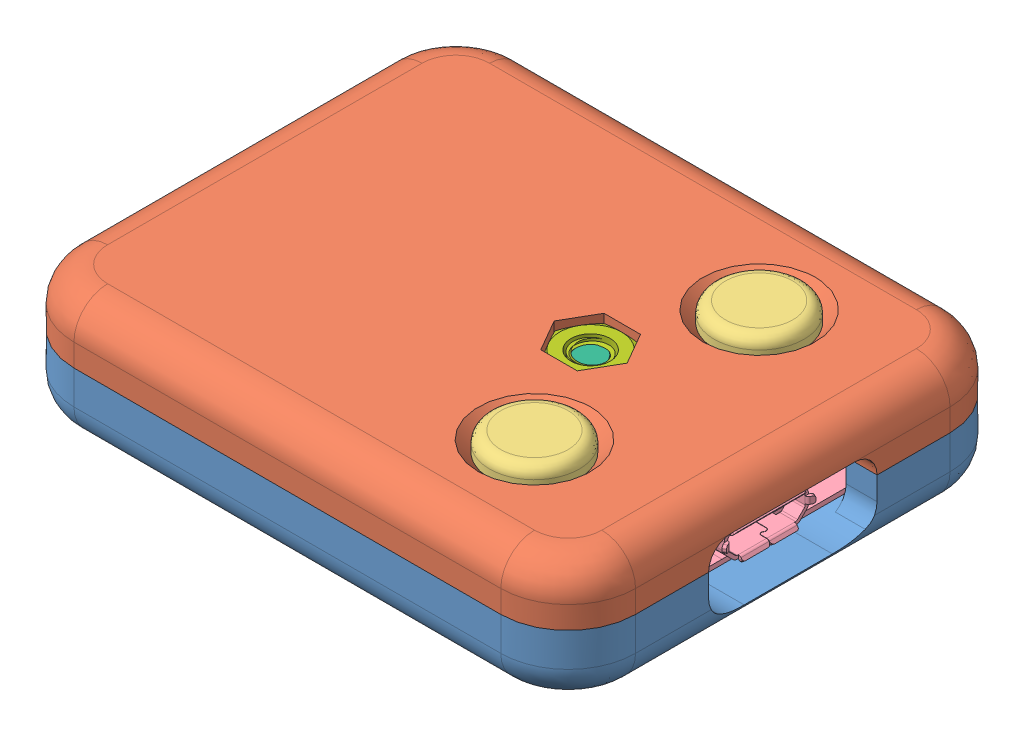
SolidWorks assembly Assem1, configuration Default. Lengths in mm.
Overall size (50 11.91 40).
7 component instances, 7 part files, 15 mates.
Components (placement in the parent):
- Base-1: Base [Default] at (22.2345 16.4906 39.6216) size (50 6 40)
- Top-1: Top [Default] at (22.2345 27.4906 39.6216) x (1 0 0) z (0 0 -1) size (50 7 40)
- Buttons-1: Buttons [Default] at (34.2345 24.2021 49.6216) x (0 0 -1) z (1 0 0) size (28 4 8)
- KeyFob-1: KeyFob [Default] at (22.2345 19.9021 39.6216) x (0 0 1) z (0 1 0) size (35.21 45.08 5.3)
- CR2032.stp-1: CR2032.stp [Default] at (11.901 23.9021 39.641) x (-0.837169 0 -0.546944) z (0 -1 0) size (20.58 20 4.09)
- Bolt-1: Bolt [     M3 X 10] at (29.2345 18.2645 39.6216) x (0.866813 0 -0.498633) z (0.498633 0 0.866813) size (6 10.32 6)
- keystone-PN4708.step-1: keystone-PN4708.step [Default] at (29.2345 24.4906 39.6216) x (-0.5 0 -0.866025) z (0.866025 0 -0.5) size (6.36 2.41 6.36)
Mates (geometry in assembly coordinates):
- Coincident2: coincident aligned: plane of Base-1 through (47.2345 22.4906 59.6216) normal (0 0 1); plane of Top-1 through (47.2345 22.4906 59.6216) normal (0 0 1)
- Coincident3: coincident aligned: plane of Base-1 through (-2.7655 22.4906 59.6216) normal (-1 0 0); plane of Top-1 through (-2.7655 22.4906 19.6216) normal (-1 0 0)
- Concentric1: concentric anti-aligned: cylinder of Top-1 through (34.2345 13.1769 49.6216) axis (0 1 0) radius 4; cylinder of Buttons-1 through (34.2345 28.2021 49.6216) axis (0 -1 0) radius 4
- Coincident6: coincident anti-aligned: circle of Top-1; cylinder of Buttons-1 through (34.2345 28.2021 29.6216) axis (0 -1 0) radius 4
- Coincident10: coincident anti-aligned: plane of Base-1 through (22.2345 22.4906 39.6216) normal (0 1 0); plane of Top-1 through (22.2345 22.4906 39.6216) normal (0 -1 0)
- Concentric2: concentric aligned: cylinder of Base-1 through (29.2345 30.9759 39.6216) axis (0 -1 0) radius 3; cylinder of KeyFob-1 through (29.2345 19.4906 39.6216) axis (0 -1 0) radius 3.25
- Parallel1: parallel anti-aligned: plane of KeyFob-1 through (38.2345 19.4906 57.2216) normal (0 0 1); plane of Base-1 through (-0.0155 22.4906 57.4216) normal (0 0 -1)
- Coincident12: coincident anti-aligned: plane of Base-1 through (22.2345 19.4906 39.6216) normal (0 1 0); plane of KeyFob-1 through (6.2345 19.4906 22.0216) normal (0 -1 0)
- Coincident13: coincident anti-aligned: plane of Buttons-1 through (34.2345 24.2021 49.6216) normal (0 -1 0); plane of KeyFob-1 through (34.2346 24.2021 28.6215) normal (0 1 0)
- Lock1: lock: unknown of KeyFob-1; unknown of CR2032.stp-1
- Concentric3: concentric anti-aligned: cylinder of Base-1 through (29.2345 11.9651 39.6216) axis (0 1 0) radius 1.6; cylinder of Bolt-1 through (29.2345 18.2645 39.6216) axis (0 -1 0) radius 1.49
- Coincident14: coincident aligned: cone of Base-1 through (29.2345 17.9906 39.6216) axis (0 1 0); cone of Bolt-1 through (29.2345 18.0906 39.6216) axis (0 1 0)
- Concentric4: concentric aligned: circle of Bolt-1; circle of keystone-PN4708.step-1
- Coincident15: coincident anti-aligned: plane of Top-1 through (22.2345 24.4906 39.6216) normal (0 1 0); plane of keystone-PN4708.step-1 through (28.3595 24.4906 38.1061) normal (0 -1 0)
- Parallel2: parallel anti-aligned: plane of Top-1 through (32.4845 24.4906 39.6216) normal (-0.866025 0 0.5); plane of keystone-PN4708.step-1 through (32.4099 26.7636 39.6216) normal (0.866025 0 -0.5)
